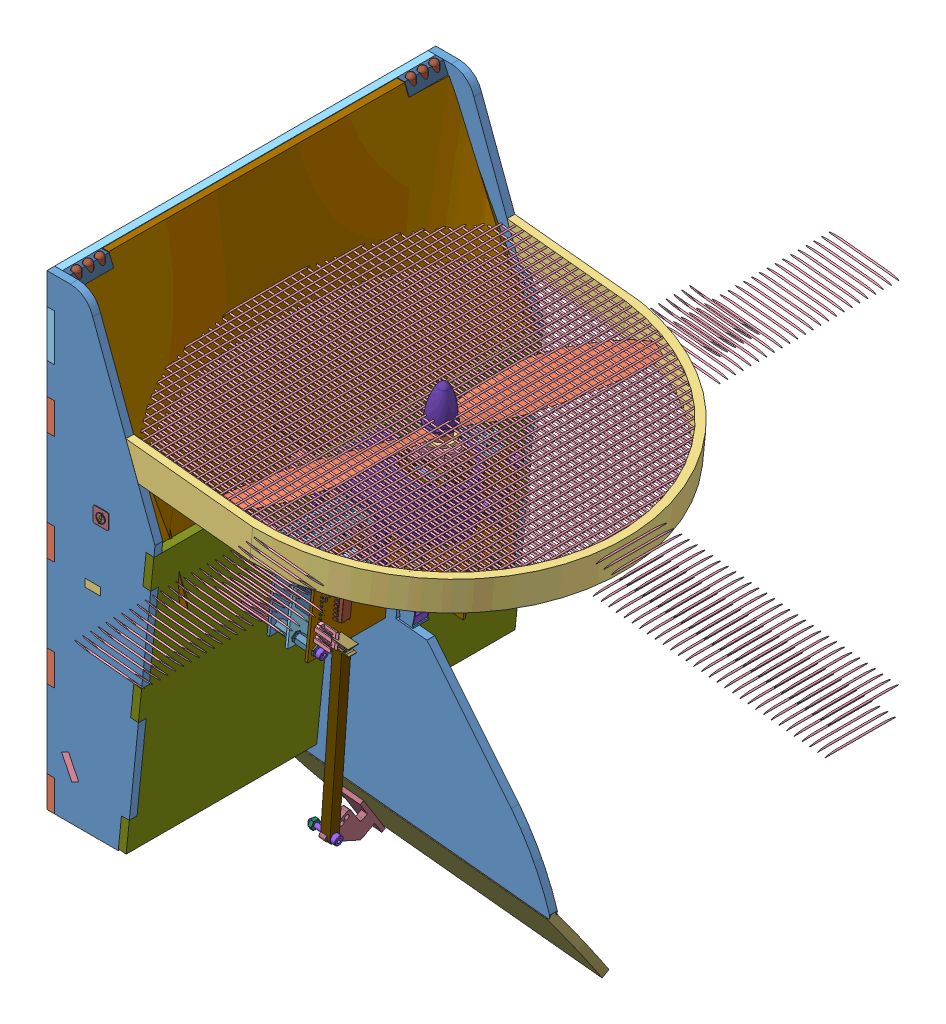
SolidWorks assembly AssTotaleSimu6, configuration Défaut. Lengths in mm. (continued)
Components (placement in the parent): (continued)
- AssStructSimu-1: AssStructSimu [Défaut] at (-125.7658 -1.8483 624.6548) x (1 0 0) z (0 0 -1) size (253.25 324.59 251.6) (continued)
  - AssProtec-1: AssProtec [Défaut] at (86.6746 190.4649 284.6351) x (0 0 -1) z (0.101852 -0.9948 0) size (250 237.46 20) (continued)
    - AssGrillage-2: AssGrillage [Défaut] at (339.6086 -132.5428 241.6839) x (0 0 1) z (-1 0 0) size (2.02 237.05 250) (continued)
      - barreau-208: barreau [Défaut] at (-0.1839 -1.5314 233.7823) x (0.998922 0 0.04641) z (0 1 0) size (1 1 400)
      - barreau-209: barreau [Défaut] at (-0.1839 -1.5314 228.7823) x (0.998922 0 0.04641) z (0 1 0) size (1 1 400)
      - barreau-210: barreau [Défaut] at (-0.1839 -1.5314 223.7823) x (0.998922 0 0.04641) z (0 1 0) size (1 1 400)
      - barreau-211: barreau [Défaut] at (-0.1839 -1.5314 218.7823) x (0.998922 0 0.04641) z (0 1 0) size (1 1 400)
      - barreau-212: barreau [Défaut] at (-0.1839 -1.5314 213.7823) x (0.998922 0 0.04641) z (0 1 0) size (1 1 400)
      - barreau-213: barreau [Défaut] at (-0.1839 -1.5314 208.7823) x (0.998922 0 0.04641) z (0 1 0) size (1 1 400)
      - barreau-214: barreau [Défaut] at (-0.1839 -1.5314 203.7823) x (0.998922 0 0.04641) z (0 1 0) size (1 1 400)
  - AssCarte-1: AssCarte [Défaut] at (38.0121 147.1029 290.772) x (-0.101852 0.9948 0) z (0.9948 0.101852 0) size (66.52 130.57 98.72)
    - carte_onduleur_v3-1: carte_onduleur_v3 [Défaut] at (-131.8199 12.0892 20.7912) size (66.52 130.57 82.34)
      - Layer_1-1: Layer_1 [Défaut] at origin size (60 130 1.61)
      - BTN-1: BTN [Défaut] at (-25.5 7.4 0.803) x (0 -1 0) z (0 0 1) size (6.76 3.64 4.37)
        - Open CASCADE STEP translator 6.8 1.2.1-1: Open CASCADE STEP translator 6.8 1.2.1 [Défaut] at origin size (6.76 3.64 4.37)
          - Body_1-1: Body_1 [Défaut] at (-0.5 -2 0) size (6.76 3.64 4.37)
            - =_[0_1_1_3]-1: =_[0_1_1_3] [Défaut] at origin size (6 3.64 4.37)
            - =_[0_1_1_4]-1: =_[0_1_1_4] [Défaut] at origin size (0.38 1 0.67)
            - =_[0_1_1_5]-1: =_[0_1_1_5] [Défaut] at origin size (0.38 1 0.67)
      - CON_IO1-1: CON_IO1 [Défaut] at (-11.3 12.1 0.803) x (0 -1 0) z (0 0 1) size (13 30 57.5)
        - Open CASCADE STEP translator 6.8 1.3.1-1: Open CASCADE STEP translator 6.8 1.3.1 [Défaut] at origin size (13 30 57.5)
          - Body_1_2-1: Body_1_2 [Défaut] at (-3 -15 8) x (0 -1 0) z (-1 0 0) size (30 57.5 13)
            - 1-1: 1 [Défaut] at origin size (30 50 1.61)
            - 10-1: 10 [Défaut] at (-14.395 31.0465 0.803) x (-1 0 0) z (0 0 1) size (5.59 6.35 1.11)
              - =_[0_1_1_4]-1: =_[0_1_1_4] [Défaut] at origin size (5.59 6.35 1.11)
                - 11-1: 11 [Défaut] at (2 3.3 0) x (-1 0 0) z (0 0 1) size (5.59 6.35 1.11)
                  - =_[0_1_1_3]_2-1: =_[0_1_1_3]_2 [Défaut] at origin size (0.44 0.55 0.36)
                  - =_[0_1_1_4]_2-1: =_[0_1_1_4]_2 [Défaut] at origin size (5.59 4.15 0.36)
                  - =_[0_1_1_5]_2-1: =_[0_1_1_5]_2 [Défaut] at origin size (5.35 6.1 1.1)
                  - =_[0_1_1_6]-1: =_[0_1_1_6] [Défaut] at origin size (0.44 0.55 0.36)
                  - =_[0_1_1_7]-1: =_[0_1_1_7] [Défaut] at origin size (0.44 0.55 0.36)
                  - =_[0_1_1_8]-1: =_[0_1_1_8] [Défaut] at origin size (0.44 0.55 0.36)
            - 13-1: 13 [Défaut] at (-12.62 16.6 -0.803) x (-1 0 0) z (0 0 -1) size (5.59 6.35 1.11)
              - =_[0_1_1_13]-1: =_[0_1_1_13] [Défaut] at origin size (5.59 6.35 1.11)
                - 11-1: 11 [Défaut] at (2 3.3 0) x (-1 0 0) z (0 0 1) size (5.59 6.35 1.11)
                  - =_[0_1_1_3]_2-1: =_[0_1_1_3]_2 [Défaut] at origin size (0.44 0.55 0.36)
                  - =_[0_1_1_4]_2-1: =_[0_1_1_4]_2 [Défaut] at origin size (5.59 4.15 0.36)
                  - =_[0_1_1_5]_2-1: =_[0_1_1_5]_2 [Défaut] at origin size (5.35 6.1 1.1)
                  - =_[0_1_1_6]-1: =_[0_1_1_6] [Défaut] at origin size (0.44 0.55 0.36)
                  - =_[0_1_1_7]-1: =_[0_1_1_7] [Défaut] at origin size (0.44 0.55 0.36)
                  - =_[0_1_1_8]-1: =_[0_1_1_8] [Défaut] at origin size (0.44 0.55 0.36)
            - 16-1: 16 [Défaut] at (-4.2 24.2 0.803) x (-1 0 0) z (0 0 1) size (12.8 0.5 13)
              - =_[0_1_1_15]-1: =_[0_1_1_15] [Défaut] at origin size (12.8 0.5 13)
                - 17-1: 17 [Défaut] at (2.7 0 0) x (1 0 0) z (0 -1 0) size (12.8 13 0.5)
            - 19-1: 19 [Défaut] at (-4.1 6.8 0.803) x (-1 0 0) z (0 0 1) size (12.8 0.5 13)
              - =_[0_1_1_18]-1: =_[0_1_1_18] [Défaut] at origin size (12.8 0.5 13)
                - 17-1: 17 [Défaut] at (2.7 0 0) x (1 0 0) z (0 -1 0) size (12.8 13 0.5)
            - 24-1: 24 [Défaut] at (-8.1 16.5 -0.803) x (0 1 0) z (0 0 -1) size (7.75 5.13 1.17)
              - =_[0_1_1_20]-1: =_[0_1_1_20] [Défaut] at origin size (7.75 5.13 1.17)
                - 20-1: 20 [Défaut] at origin size (7.59 5.13 1.07)
                - 21-1: 21 [Défaut] at (-14.478 0 0) x (-1 0 0) z (0 0 1) size (0.76 5.08 1.17)
                - 22-1: 22 [Défaut] at origin size (0.76 5.08 1.17)
            - 35-1: 35 [Défaut] at (-25.3 25.5 0.803) x (0 -1 0) z (0 0 1) size (6.05 5.2 1.7)
              - =_[0_1_1_25]-1: =_[0_1_1_25] [Défaut] at origin size (6.05 5.2 1.7)
                - 25-1: 25 [Défaut] at origin size (4.3 5.2 1.53)
                - 26-1: 26 [Défaut] at origin size (0.88 0.51 1.06)
                - 27-1: 27 [Défaut] at origin size (0.88 0.51 1.06)
                - 28-1: 28 [Défaut] at origin size (0.88 0.51 1.06)
                - 29-1: 29 [Défaut] at origin size (0.88 0.51 1.06)
                - 30-1: 30 [Défaut] at (11.6 -5.08 0) x (-1 0 0) z (0 0 1) size (0.87 0.51 1.06)
                - 31-1: 31 [Défaut] at (11.6 -2.54 0) x (-1 0 0) z (0 0 1) size (0.87 0.51 1.06)
                - 32-1: 32 [Défaut] at (11.6 0 0) x (-1 0 0) z (0 0 1) size (0.87 0.51 1.06)
                - 33-1: 33 [Défaut] at (11.6 2.54 0) x (-1 0 0) z (0 0 1) size (0.87 0.51 1.06)
            - 40-1: 40 [Défaut] at (-27.6 27.2 0.803) size (2.34 1.04 0.5)
              - =_[0_1_1_36]-1: =_[0_1_1_36] [Défaut] at origin size (2.34 1.04 0.5)
                - 36-1: 36 [Défaut] at origin size (2.29 1.04 0.43)
                - 37-1: 37 [Défaut] at (0.3048 0 0) x (-1 0 0) z (0 0 1) size (0.51 1.02 0.5)
                - 38-1: 38 [Défaut] at origin size (0.51 1.02 0.5)
            - 42-1: 42 [Défaut] at (-22.1 21.6 0.803) x (0 1 0) z (0 0 1) size (2.34 1.04 0.5)
              - =_[0_1_1_36]-1: =_[0_1_1_36] [Défaut] at origin size (2.34 1.04 0.5)
                - 36-1: 36 [Défaut] at origin size (2.29 1.04 0.43)
                - 37-1: 37 [Défaut] at (0.3048 0 0) x (-1 0 0) z (0 0 1) size (0.51 1.02 0.5)
                - 38-1: 38 [Défaut] at origin size (0.51 1.02 0.5)
            - 47-1: 47 [Défaut] at (-14.7664 14.5 -0.803) x (-1 0 0) z (0 0 -1) size (2.34 1.04 0.5)
              - =_[0_1_1_42]-1: =_[0_1_1_42] [Défaut] at origin size (2.34 1.04 0.5)
                - 43-1: 43 [Défaut] at origin size (2.29 1.04 0.43)
                - 44-1: 44 [Défaut] at (0.3048 0 0) x (-1 0 0) z (0 0 1) size (0.51 1.02 0.5)
                - 45-1: 45 [Défaut] at origin size (0.51 1.02 0.5)
            - 57-1: 57 [Défaut] at (-15.3 2.7 -0.803) x (0 -1 0) z (0 0 -1) size (10.36 15.24 6.14)
              - =_[0_1_1_47]-1: =_[0_1_1_47] [Défaut] at origin size (10.36 15.24 6.14)
                - 55-1: 55 [Défaut] at (1.8 -1.2 3) x (1 0 0) z (0 1 0) size (10.36 6.14 15.24)
                  - 54-1: 54 [Défaut] at origin size (10.36 6.14 7.62)
                    - 52-1: 52 [Défaut] at origin size (10.36 6.14 2.54)
                      - 48-1: 48 [Défaut] at origin size (8.4 2.54 2.54)
                      - 49-1: 49 [Défaut] at (-0.0461 1.2682 1.27) x (0 0 -1) z (0.999998 -0.002105 0) size (1.95 5.07 7.58)
                    - 52-2: 52 [Défaut] at (0 0 -2.54) size (10.36 6.14 2.54)
                      - 48-1: 48 [Défaut] at origin size (8.4 2.54 2.54)
                      - 49-1: 49 [Défaut] at (-0.0461 1.2682 1.27) x (0 0 -1) z (0.999998 -0.002105 0) size (1.95 5.07 7.58)
                    - 52-3: 52 [Défaut] at (0 0 -5.08) size (10.36 6.14 2.54)
                      - 48-1: 48 [Défaut] at origin size (8.4 2.54 2.54)
                      - 49-1: 49 [Défaut] at (-0.0461 1.2682 1.27) x (0 0 -1) z (0.999998 -0.002105 0) size (1.95 5.07 7.58)
                  - 54-2: 54 [Défaut] at (0 0 -7.62) size (10.36 6.14 7.62)
                    - 52-1: 52 [Défaut] at origin size (10.36 6.14 2.54)
                      - 48-1: 48 [Défaut] at origin size (8.4 2.54 2.54)
                      - 49-1: 49 [Défaut] at (-0.0461 1.2682 1.27) x (0 0 -1) z (0.999998 -0.002105 0) size (1.95 5.07 7.58)
                    - 52-2: 52 [Défaut] at (0 0 -2.54) size (10.36 6.14 2.54)
                      - 48-1: 48 [Défaut] at origin size (8.4 2.54 2.54)
                      - 49-1: 49 [Défaut] at (-0.0461 1.2682 1.27) x (0 0 -1) z (0.999998 -0.002105 0) size (1.95 5.07 7.58)
                    - 52-3: 52 [Défaut] at (0 0 -5.08) size (10.36 6.14 2.54)
                      - 48-1: 48 [Défaut] at origin size (8.4 2.54 2.54)
                      - 49-1: 49 [Défaut] at (-0.0461 1.2682 1.27) x (0 0 -1) z (0.999998 -0.002105 0) size (1.95 5.07 7.58)
            - 59-1: 59 [Défaut] at (-26.5 31 0.803) x (0 -1 0) z (0 0 1) size (2.34 1.04 0.5)
              - =_[0_1_1_42]-1: =_[0_1_1_42] [Défaut] at origin size (2.34 1.04 0.5)
                - 43-1: 43 [Défaut] at origin size (2.29 1.04 0.43)
                - 44-1: 44 [Défaut] at (0.3048 0 0) x (-1 0 0) z (0 0 1) size (0.51 1.02 0.5)
                - 45-1: 45 [Défaut] at origin size (0.51 1.02 0.5)
            - 61-1: 61 [Défaut] at (-21.6 17.8 0.803) x (-1 0 0) z (0 0 1) size (2.34 1.04 0.5)
              - =_[0_1_1_42]-1: =_[0_1_1_42] [Défaut] at origin size (2.34 1.04 0.5)
                - 43-1: 43 [Défaut] at origin size (2.29 1.04 0.43)
                - 44-1: 44 [Défaut] at (0.3048 0 0) x (-1 0 0) z (0 0 1) size (0.51 1.02 0.5)
                - 45-1: 45 [Défaut] at origin size (0.51 1.02 0.5)
            - 74-1: 74 [Défaut] at (-4.9 41.8 0.803) x (0 -1 0) z (0 0 1) size (6 4.9 1.75)
              - =_[0_1_1_56]-1: =_[0_1_1_56] [Défaut] at origin size (6 4.9 1.75)
                - 72-1: 72 [Défaut] at origin size (6 4.9 1.75)
                  - =_[0_1_1_2]-1: =_[0_1_1_2] [Défaut] at origin size (3.9 4.9 1.57)
                  - =_[0_1_1_3]-1: =_[0_1_1_3] [Défaut] at origin size (6 4.22 1)
                    - =_[0_1_1_60]-1: =_[0_1_1_60] [Défaut] at origin size (1.05 0.41 1)
                    - =_[0_1_1_61]-1: =_[0_1_1_61] [Défaut] at origin size (1.05 0.41 1)
                    - =_[0_1_1_62]-1: =_[0_1_1_62] [Défaut] at origin size (1.05 0.41 1)
                    - =_[0_1_1_63]-1: =_[0_1_1_63] [Défaut] at origin size (1.05 0.41 1)
                    - =_[0_1_1_64]-1: =_[0_1_1_64] [Défaut] at origin size (1.05 0.41 1)
                    - =_[0_1_1_65]-1: =_[0_1_1_65] [Défaut] at origin size (1.05 0.41 1)
                    - =_[0_1_1_66]-1: =_[0_1_1_66] [Défaut] at origin size (1.05 0.41 1)
                    - =_[0_1_1_67]-1: =_[0_1_1_67] [Défaut] at origin size (1.05 0.41 1)
            - 76-1: 76 [Défaut] at (-8.5 40.5664 0.803) x (0 1 0) z (0 0 1) size (2.34 1.04 0.5)
              - =_[0_1_1_42]-1: =_[0_1_1_42] [Défaut] at origin size (2.34 1.04 0.5)
                - 43-1: 43 [Défaut] at origin size (2.29 1.04 0.43)
                - 44-1: 44 [Défaut] at (0.3048 0 0) x (-1 0 0) z (0 0 1) size (0.51 1.02 0.5)
                - 45-1: 45 [Défaut] at origin size (0.51 1.02 0.5)
            - 78-1: 78 [Défaut] at (-5.9 46.4 0.803) x (-1 0 0) z (0 0 1) size (2.34 1.04 0.5)
              - =_[0_1_1_42]-1: =_[0_1_1_42] [Défaut] at origin size (2.34 1.04 0.5)
                - 43-1: 43 [Défaut] at origin size (2.29 1.04 0.43)
                - 44-1: 44 [Défaut] at (0.3048 0 0) x (-1 0 0) z (0 0 1) size (0.51 1.02 0.5)
                - 45-1: 45 [Défaut] at origin size (0.51 1.02 0.5)
            - 80-1: 80 [Défaut] at (-7 48.1 0.803) size (2.34 1.04 0.5)
              - =_[0_1_1_42]-1: =_[0_1_1_42] [Défaut] at origin size (2.34 1.04 0.5)
                - 43-1: 43 [Défaut] at origin size (2.29 1.04 0.43)
                - 44-1: 44 [Défaut] at (0.3048 0 0) x (-1 0 0) z (0 0 1) size (0.51 1.02 0.5)
                - 45-1: 45 [Défaut] at origin size (0.51 1.02 0.5)
            - 82-1: 82 [Défaut] at (-6 37.1 0.803) size (2.34 1.04 0.5)
              - =_[0_1_1_42]-1: =_[0_1_1_42] [Défaut] at origin size (2.34 1.04 0.5)
                - 43-1: 43 [Défaut] at origin size (2.29 1.04 0.43)
                - 44-1: 44 [Défaut] at (0.3048 0 0) x (-1 0 0) z (0 0 1) size (0.51 1.02 0.5)
                - 45-1: 45 [Défaut] at origin size (0.51 1.02 0.5)
      - CON_IO2-1: CON_IO2 [Défaut] at (-11.3 -2.7 0.803) x (0 -1 0) z (0 0 1) size (13 30 57.5)
        - Open CASCADE STEP translator 6.8 1.4.1-1: Open CASCADE STEP translator 6.8 1.4.1 [Défaut] at origin size (13 30 57.5)
          - Body_1_2-1: Body_1_2 [Défaut] at (-3 -15 8) x (0 -1 0) z (-1 0 0) size (30 57.5 13)
            - 1-1: 1 [Défaut] at origin size (30 50 1.61)
            - 10-1: 10 [Défaut] at (-14.395 31.0465 0.803) x (-1 0 0) z (0 0 1) size (5.59 6.35 1.11)
              - =_[0_1_1_4]-1: =_[0_1_1_4] [Défaut] at origin size (5.59 6.35 1.11)
                - 11-1: 11 [Défaut] at (2 3.3 0) x (-1 0 0) z (0 0 1) size (5.59 6.35 1.11)
                  - =_[0_1_1_3]_2-1: =_[0_1_1_3]_2 [Défaut] at origin size (0.44 0.55 0.36)
                  - =_[0_1_1_4]_2-1: =_[0_1_1_4]_2 [Défaut] at origin size (5.59 4.15 0.36)
                  - =_[0_1_1_5]_2-1: =_[0_1_1_5]_2 [Défaut] at origin size (5.35 6.1 1.1)
                  - =_[0_1_1_6]-1: =_[0_1_1_6] [Défaut] at origin size (0.44 0.55 0.36)
                  - =_[0_1_1_7]-1: =_[0_1_1_7] [Défaut] at origin size (0.44 0.55 0.36)
                  - =_[0_1_1_8]-1: =_[0_1_1_8] [Défaut] at origin size (0.44 0.55 0.36)
            - 13-1: 13 [Défaut] at (-12.62 16.6 -0.803) x (-1 0 0) z (0 0 -1) size (5.59 6.35 1.11)
              - =_[0_1_1_13]-1: =_[0_1_1_13] [Défaut] at origin size (5.59 6.35 1.11)
                - 11-1: 11 [Défaut] at (2 3.3 0) x (-1 0 0) z (0 0 1) size (5.59 6.35 1.11)
                  - =_[0_1_1_3]_2-1: =_[0_1_1_3]_2 [Défaut] at origin size (0.44 0.55 0.36)
                  - =_[0_1_1_4]_2-1: =_[0_1_1_4]_2 [Défaut] at origin size (5.59 4.15 0.36)
                  - =_[0_1_1_5]_2-1: =_[0_1_1_5]_2 [Défaut] at origin size (5.35 6.1 1.1)
                  - =_[0_1_1_6]-1: =_[0_1_1_6] [Défaut] at origin size (0.44 0.55 0.36)
                  - =_[0_1_1_7]-1: =_[0_1_1_7] [Défaut] at origin size (0.44 0.55 0.36)
                  - =_[0_1_1_8]-1: =_[0_1_1_8] [Défaut] at origin size (0.44 0.55 0.36)
            - 16-1: 16 [Défaut] at (-4.2 24.2 0.803) x (-1 0 0) z (0 0 1) size (12.8 0.5 13)
              - =_[0_1_1_15]-1: =_[0_1_1_15] [Défaut] at origin size (12.8 0.5 13)
                - 17-1: 17 [Défaut] at (2.7 0 0) x (1 0 0) z (0 -1 0) size (12.8 13 0.5)
            - 19-1: 19 [Défaut] at (-4.1 6.8 0.803) x (-1 0 0) z (0 0 1) size (12.8 0.5 13)
              - =_[0_1_1_18]-1: =_[0_1_1_18] [Défaut] at origin size (12.8 0.5 13)
                - 17-1: 17 [Défaut] at (2.7 0 0) x (1 0 0) z (0 -1 0) size (12.8 13 0.5)
            - 24-1: 24 [Défaut] at (-8.1 16.5 -0.803) x (0 1 0) z (0 0 -1) size (7.75 5.13 1.17)
              - =_[0_1_1_20]-1: =_[0_1_1_20] [Défaut] at origin size (7.75 5.13 1.17)
                - 20-1: 20 [Défaut] at origin size (7.59 5.13 1.07)
                - 21-1: 21 [Défaut] at (-14.478 0 0) x (-1 0 0) z (0 0 1) size (0.76 5.08 1.17)
                - 22-1: 22 [Défaut] at origin size (0.76 5.08 1.17)
            - 35-1: 35 [Défaut] at (-25.3 25.5 0.803) x (0 -1 0) z (0 0 1) size (6.05 5.2 1.7)
              - =_[0_1_1_25]-1: =_[0_1_1_25] [Défaut] at origin size (6.05 5.2 1.7)
                - 25-1: 25 [Défaut] at origin size (4.3 5.2 1.53)
                - 26-1: 26 [Défaut] at origin size (0.88 0.51 1.06)
                - 27-1: 27 [Défaut] at origin size (0.88 0.51 1.06)
                - 28-1: 28 [Défaut] at origin size (0.88 0.51 1.06)
                - 29-1: 29 [Défaut] at origin size (0.88 0.51 1.06)
                - 30-1: 30 [Défaut] at (11.6 -5.08 0) x (-1 0 0) z (0 0 1) size (0.87 0.51 1.06)
                - 31-1: 31 [Défaut] at (11.6 -2.54 0) x (-1 0 0) z (0 0 1) size (0.87 0.51 1.06)
                - 32-1: 32 [Défaut] at (11.6 0 0) x (-1 0 0) z (0 0 1) size (0.87 0.51 1.06)
                - 33-1: 33 [Défaut] at (11.6 2.54 0) x (-1 0 0) z (0 0 1) size (0.87 0.51 1.06)
            - 40-1: 40 [Défaut] at (-27.6 27.2 0.803) size (2.34 1.04 0.5)
              - =_[0_1_1_36]-1: =_[0_1_1_36] [Défaut] at origin size (2.34 1.04 0.5)
                - 36-1: 36 [Défaut] at origin size (2.29 1.04 0.43)
                - 37-1: 37 [Défaut] at (0.3048 0 0) x (-1 0 0) z (0 0 1) size (0.51 1.02 0.5)
                - 38-1: 38 [Défaut] at origin size (0.51 1.02 0.5)
            - 42-1: 42 [Défaut] at (-22.1 21.6 0.803) x (0 1 0) z (0 0 1) size (2.34 1.04 0.5)
              - =_[0_1_1_36]-1: =_[0_1_1_36] [Défaut] at origin size (2.34 1.04 0.5)
                - 36-1: 36 [Défaut] at origin size (2.29 1.04 0.43)
                - 37-1: 37 [Défaut] at (0.3048 0 0) x (-1 0 0) z (0 0 1) size (0.51 1.02 0.5)
                - 38-1: 38 [Défaut] at origin size (0.51 1.02 0.5)
            - 47-1: 47 [Défaut] at (-14.7664 14.5 -0.803) x (-1 0 0) z (0 0 -1) size (2.34 1.04 0.5)
              - =_[0_1_1_42]-1: =_[0_1_1_42] [Défaut] at origin size (2.34 1.04 0.5)
                - 43-1: 43 [Défaut] at origin size (2.29 1.04 0.43)
                - 44-1: 44 [Défaut] at (0.3048 0 0) x (-1 0 0) z (0 0 1) size (0.51 1.02 0.5)
                - 45-1: 45 [Défaut] at origin size (0.51 1.02 0.5)
            - 57-1: 57 [Défaut] at (-15.3 2.7 -0.803) x (0 -1 0) z (0 0 -1) size (10.36 15.24 6.14)
              - =_[0_1_1_47]-1: =_[0_1_1_47] [Défaut] at origin size (10.36 15.24 6.14)
                - 55-1: 55 [Défaut] at (1.8 -1.2 3) x (1 0 0) z (0 1 0) size (10.36 6.14 15.24)
                  - 54-1: 54 [Défaut] at origin size (10.36 6.14 7.62)
                    - 52-1: 52 [Défaut] at origin size (10.36 6.14 2.54)
                      - 48-1: 48 [Défaut] at origin size (8.4 2.54 2.54)
                      - 49-1: 49 [Défaut] at (-0.0461 1.2682 1.27) x (0 0 -1) z (0.999998 -0.002105 0) size (1.95 5.07 7.58)
                    - 52-2: 52 [Défaut] at (0 0 -2.54) size (10.36 6.14 2.54)
                      - 48-1: 48 [Défaut] at origin size (8.4 2.54 2.54)
                      - 49-1: 49 [Défaut] at (-0.0461 1.2682 1.27) x (0 0 -1) z (0.999998 -0.002105 0) size (1.95 5.07 7.58)
                    - 52-3: 52 [Défaut] at (0 0 -5.08) size (10.36 6.14 2.54)
                      - 48-1: 48 [Défaut] at origin size (8.4 2.54 2.54)
                      - 49-1: 49 [Défaut] at (-0.0461 1.2682 1.27) x (0 0 -1) z (0.999998 -0.002105 0) size (1.95 5.07 7.58)
                  - 54-2: 54 [Défaut] at (0 0 -7.62) size (10.36 6.14 7.62)
                    - 52-1: 52 [Défaut] at origin size (10.36 6.14 2.54)
                      - 48-1: 48 [Défaut] at origin size (8.4 2.54 2.54)
                      - 49-1: 49 [Défaut] at (-0.0461 1.2682 1.27) x (0 0 -1) z (0.999998 -0.002105 0) size (1.95 5.07 7.58)
                    - 52-2: 52 [Défaut] at (0 0 -2.54) size (10.36 6.14 2.54)
                      - 48-1: 48 [Défaut] at origin size (8.4 2.54 2.54)
                      - 49-1: 49 [Défaut] at (-0.0461 1.2682 1.27) x (0 0 -1) z (0.999998 -0.002105 0) size (1.95 5.07 7.58)
                    - 52-3: 52 [Défaut] at (0 0 -5.08) size (10.36 6.14 2.54)
                      - 48-1: 48 [Défaut] at origin size (8.4 2.54 2.54)
                      - 49-1: 49 [Défaut] at (-0.0461 1.2682 1.27) x (0 0 -1) z (0.999998 -0.002105 0) size (1.95 5.07 7.58)
            - 59-1: 59 [Défaut] at (-26.5 31 0.803) x (0 -1 0) z (0 0 1) size (2.34 1.04 0.5)
              - =_[0_1_1_42]-1: =_[0_1_1_42] [Défaut] at origin size (2.34 1.04 0.5)
                - 43-1: 43 [Défaut] at origin size (2.29 1.04 0.43)
                - 44-1: 44 [Défaut] at (0.3048 0 0) x (-1 0 0) z (0 0 1) size (0.51 1.02 0.5)
                - 45-1: 45 [Défaut] at origin size (0.51 1.02 0.5)
            - 61-1: 61 [Défaut] at (-21.6 17.8 0.803) x (-1 0 0) z (0 0 1) size (2.34 1.04 0.5)
              - =_[0_1_1_42]-1: =_[0_1_1_42] [Défaut] at origin size (2.34 1.04 0.5)
                - 43-1: 43 [Défaut] at origin size (2.29 1.04 0.43)
                - 44-1: 44 [Défaut] at (0.3048 0 0) x (-1 0 0) z (0 0 1) size (0.51 1.02 0.5)
                - 45-1: 45 [Défaut] at origin size (0.51 1.02 0.5)
            - 74-1: 74 [Défaut] at (-4.9 41.8 0.803) x (0 -1 0) z (0 0 1) size (6 4.9 1.75)
              - =_[0_1_1_56]-1: =_[0_1_1_56] [Défaut] at origin size (6 4.9 1.75)
                - 72-1: 72 [Défaut] at origin size (6 4.9 1.75)
                  - =_[0_1_1_2]-1: =_[0_1_1_2] [Défaut] at origin size (3.9 4.9 1.57)
                  - =_[0_1_1_3]-1: =_[0_1_1_3] [Défaut] at origin size (6 4.22 1)
                    - =_[0_1_1_60]-1: =_[0_1_1_60] [Défaut] at origin size (1.05 0.41 1)
                    - =_[0_1_1_61]-1: =_[0_1_1_61] [Défaut] at origin size (1.05 0.41 1)
                    - =_[0_1_1_62]-1: =_[0_1_1_62] [Défaut] at origin size (1.05 0.41 1)
                    - =_[0_1_1_63]-1: =_[0_1_1_63] [Défaut] at origin size (1.05 0.41 1)
                    - =_[0_1_1_64]-1: =_[0_1_1_64] [Défaut] at origin size (1.05 0.41 1)
                    - =_[0_1_1_65]-1: =_[0_1_1_65] [Défaut] at origin size (1.05 0.41 1)
                    - =_[0_1_1_66]-1: =_[0_1_1_66] [Défaut] at origin size (1.05 0.41 1)
                    - =_[0_1_1_67]-1: =_[0_1_1_67] [Défaut] at origin size (1.05 0.41 1)
            - 76-1: 76 [Défaut] at (-8.5 40.5664 0.803) x (0 1 0) z (0 0 1) size (2.34 1.04 0.5)
              - =_[0_1_1_42]-1: =_[0_1_1_42] [Défaut] at origin size (2.34 1.04 0.5)
                - 43-1: 43 [Défaut] at origin size (2.29 1.04 0.43)
                - 44-1: 44 [Défaut] at (0.3048 0 0) x (-1 0 0) z (0 0 1) size (0.51 1.02 0.5)
                - 45-1: 45 [Défaut] at origin size (0.51 1.02 0.5)
            - 78-1: 78 [Défaut] at (-5.9 46.4 0.803) x (-1 0 0) z (0 0 1) size (2.34 1.04 0.5)
              - =_[0_1_1_42]-1: =_[0_1_1_42] [Défaut] at origin size (2.34 1.04 0.5)
                - 43-1: 43 [Défaut] at origin size (2.29 1.04 0.43)
                - 44-1: 44 [Défaut] at (0.3048 0 0) x (-1 0 0) z (0 0 1) size (0.51 1.02 0.5)
                - 45-1: 45 [Défaut] at origin size (0.51 1.02 0.5)
            - 80-1: 80 [Défaut] at (-7 48.1 0.803) size (2.34 1.04 0.5)
              - =_[0_1_1_42]-1: =_[0_1_1_42] [Défaut] at origin size (2.34 1.04 0.5)
                - 43-1: 43 [Défaut] at origin size (2.29 1.04 0.43)
                - 44-1: 44 [Défaut] at (0.3048 0 0) x (-1 0 0) z (0 0 1) size (0.51 1.02 0.5)
                - 45-1: 45 [Défaut] at origin size (0.51 1.02 0.5)
            - 82-1: 82 [Défaut] at (-6 37.1 0.803) size (2.34 1.04 0.5)
              - =_[0_1_1_42]-1: =_[0_1_1_42] [Défaut] at origin size (2.34 1.04 0.5)
                - 43-1: 43 [Défaut] at origin size (2.29 1.04 0.43)
                - 44-1: 44 [Défaut] at (0.3048 0 0) x (-1 0 0) z (0 0 1) size (0.51 1.02 0.5)
                - 45-1: 45 [Défaut] at origin size (0.51 1.02 0.5)
      - CON_IO3-1: CON_IO3 [Défaut] at (-11.3 -17.7 0.803) x (0 -1 0) z (0 0 1) size (13 30 57.5)
        - Open CASCADE STEP translator 6.8 1.5.1-1: Open CASCADE STEP translator 6.8 1.5.1 [Défaut] at origin size (13 30 57.5)
          - Body_1_2-1: Body_1_2 [Défaut] at (-3 -15 8) x (0 -1 0) z (-1 0 0) size (30 57.5 13)
            - 1-1: 1 [Défaut] at origin size (30 50 1.61)
            - 10-1: 10 [Défaut] at (-14.395 31.0465 0.803) x (-1 0 0) z (0 0 1) size (5.59 6.35 1.11)
              - =_[0_1_1_4]-1: =_[0_1_1_4] [Défaut] at origin size (5.59 6.35 1.11)
                - 11-1: 11 [Défaut] at (2 3.3 0) x (-1 0 0) z (0 0 1) size (5.59 6.35 1.11)
                  - =_[0_1_1_3]_2-1: =_[0_1_1_3]_2 [Défaut] at origin size (0.44 0.55 0.36)
                  - =_[0_1_1_4]_2-1: =_[0_1_1_4]_2 [Défaut] at origin size (5.59 4.15 0.36)
                  - =_[0_1_1_5]_2-1: =_[0_1_1_5]_2 [Défaut] at origin size (5.35 6.1 1.1)
                  - =_[0_1_1_6]-1: =_[0_1_1_6] [Défaut] at origin size (0.44 0.55 0.36)
                  - =_[0_1_1_7]-1: =_[0_1_1_7] [Défaut] at origin size (0.44 0.55 0.36)
                  - =_[0_1_1_8]-1: =_[0_1_1_8] [Défaut] at origin size (0.44 0.55 0.36)
            - 13-1: 13 [Défaut] at (-12.62 16.6 -0.803) x (-1 0 0) z (0 0 -1) size (5.59 6.35 1.11)
              - =_[0_1_1_13]-1: =_[0_1_1_13] [Défaut] at origin size (5.59 6.35 1.11)
                - 11-1: 11 [Défaut] at (2 3.3 0) x (-1 0 0) z (0 0 1) size (5.59 6.35 1.11)
                  - =_[0_1_1_3]_2-1: =_[0_1_1_3]_2 [Défaut] at origin size (0.44 0.55 0.36)
                  - =_[0_1_1_4]_2-1: =_[0_1_1_4]_2 [Défaut] at origin size (5.59 4.15 0.36)
                  - =_[0_1_1_5]_2-1: =_[0_1_1_5]_2 [Défaut] at origin size (5.35 6.1 1.1)
                  - =_[0_1_1_6]-1: =_[0_1_1_6] [Défaut] at origin size (0.44 0.55 0.36)
                  - =_[0_1_1_7]-1: =_[0_1_1_7] [Défaut] at origin size (0.44 0.55 0.36)
                  - =_[0_1_1_8]-1: =_[0_1_1_8] [Défaut] at origin size (0.44 0.55 0.36)
            - 16-1: 16 [Défaut] at (-4.2 24.2 0.803) x (-1 0 0) z (0 0 1) size (12.8 0.5 13)
              - =_[0_1_1_15]-1: =_[0_1_1_15] [Défaut] at origin size (12.8 0.5 13)
                - 17-1: 17 [Défaut] at (2.7 0 0) x (1 0 0) z (0 -1 0) size (12.8 13 0.5)
            - 19-1: 19 [Défaut] at (-4.1 6.8 0.803) x (-1 0 0) z (0 0 1) size (12.8 0.5 13)
              - =_[0_1_1_18]-1: =_[0_1_1_18] [Défaut] at origin size (12.8 0.5 13)
                - 17-1: 17 [Défaut] at (2.7 0 0) x (1 0 0) z (0 -1 0) size (12.8 13 0.5)
            - 24-1: 24 [Défaut] at (-8.1 16.5 -0.803) x (0 1 0) z (0 0 -1) size (7.75 5.13 1.17)
              - =_[0_1_1_20]-1: =_[0_1_1_20] [Défaut] at origin size (7.75 5.13 1.17)
                - 20-1: 20 [Défaut] at origin size (7.59 5.13 1.07)
                - 21-1: 21 [Défaut] at (-14.478 0 0) x (-1 0 0) z (0 0 1) size (0.76 5.08 1.17)
                - 22-1: 22 [Défaut] at origin size (0.76 5.08 1.17)
            - 35-1: 35 [Défaut] at (-25.3 25.5 0.803) x (0 -1 0) z (0 0 1) size (6.05 5.2 1.7)
              - =_[0_1_1_25]-1: =_[0_1_1_25] [Défaut] at origin size (6.05 5.2 1.7)
                - 25-1: 25 [Défaut] at origin size (4.3 5.2 1.53)
                - 26-1: 26 [Défaut] at origin size (0.88 0.51 1.06)
                - 27-1: 27 [Défaut] at origin size (0.88 0.51 1.06)
                - 28-1: 28 [Défaut] at origin size (0.88 0.51 1.06)
                - 29-1: 29 [Défaut] at origin size (0.88 0.51 1.06)
                - 30-1: 30 [Défaut] at (11.6 -5.08 0) x (-1 0 0) z (0 0 1) size (0.87 0.51 1.06)
                - 31-1: 31 [Défaut] at (11.6 -2.54 0) x (-1 0 0) z (0 0 1) size (0.87 0.51 1.06)
                - 32-1: 32 [Défaut] at (11.6 0 0) x (-1 0 0) z (0 0 1) size (0.87 0.51 1.06)
                - 33-1: 33 [Défaut] at (11.6 2.54 0) x (-1 0 0) z (0 0 1) size (0.87 0.51 1.06)
            - 40-1: 40 [Défaut] at (-27.6 27.2 0.803) size (2.34 1.04 0.5)
              - =_[0_1_1_36]-1: =_[0_1_1_36] [Défaut] at origin size (2.34 1.04 0.5)
                - 36-1: 36 [Défaut] at origin size (2.29 1.04 0.43)
                - 37-1: 37 [Défaut] at (0.3048 0 0) x (-1 0 0) z (0 0 1) size (0.51 1.02 0.5)
                - 38-1: 38 [Défaut] at origin size (0.51 1.02 0.5)
            - 42-1: 42 [Défaut] at (-22.1 21.6 0.803) x (0 1 0) z (0 0 1) size (2.34 1.04 0.5)
              - =_[0_1_1_36]-1: =_[0_1_1_36] [Défaut] at origin size (2.34 1.04 0.5)
                - 36-1: 36 [Défaut] at origin size (2.29 1.04 0.43)
                - 37-1: 37 [Défaut] at (0.3048 0 0) x (-1 0 0) z (0 0 1) size (0.51 1.02 0.5)
                - 38-1: 38 [Défaut] at origin size (0.51 1.02 0.5)
            - 47-1: 47 [Défaut] at (-14.7664 14.5 -0.803) x (-1 0 0) z (0 0 -1) size (2.34 1.04 0.5)
              - =_[0_1_1_42]-1: =_[0_1_1_42] [Défaut] at origin size (2.34 1.04 0.5)
                - 43-1: 43 [Défaut] at origin size (2.29 1.04 0.43)
                - 44-1: 44 [Défaut] at (0.3048 0 0) x (-1 0 0) z (0 0 1) size (0.51 1.02 0.5)
                - 45-1: 45 [Défaut] at origin size (0.51 1.02 0.5)
            - 57-1: 57 [Défaut] at (-15.3 2.7 -0.803) x (0 -1 0) z (0 0 -1) size (10.36 15.24 6.14)
              - =_[0_1_1_47]-1: =_[0_1_1_47] [Défaut] at origin size (10.36 15.24 6.14)
                - 55-1: 55 [Défaut] at (1.8 -1.2 3) x (1 0 0) z (0 1 0) size (10.36 6.14 15.24)
                  - 54-1: 54 [Défaut] at origin size (10.36 6.14 7.62)
                    - 52-1: 52 [Défaut] at origin size (10.36 6.14 2.54)
                      - 48-1: 48 [Défaut] at origin size (8.4 2.54 2.54)
                      - 49-1: 49 [Défaut] at (-0.0461 1.2682 1.27) x (0 0 -1) z (0.999998 -0.002105 0) size (1.95 5.07 7.58)
                    - 52-2: 52 [Défaut] at (0 0 -2.54) size (10.36 6.14 2.54)
                      - 48-1: 48 [Défaut] at origin size (8.4 2.54 2.54)
                      - 49-1: 49 [Défaut] at (-0.0461 1.2682 1.27) x (0 0 -1) z (0.999998 -0.002105 0) size (1.95 5.07 7.58)
                    - 52-3: 52 [Défaut] at (0 0 -5.08) size (10.36 6.14 2.54)
                      - 48-1: 48 [Défaut] at origin size (8.4 2.54 2.54)
                      - 49-1: 49 [Défaut] at (-0.0461 1.2682 1.27) x (0 0 -1) z (0.999998 -0.002105 0) size (1.95 5.07 7.58)
                  - 54-2: 54 [Défaut] at (0 0 -7.62) size (10.36 6.14 7.62)
                    - 52-1: 52 [Défaut] at origin size (10.36 6.14 2.54)
                      - 48-1: 48 [Défaut] at origin size (8.4 2.54 2.54)
                      - 49-1: 49 [Défaut] at (-0.0461 1.2682 1.27) x (0 0 -1) z (0.999998 -0.002105 0) size (1.95 5.07 7.58)
                    - 52-2: 52 [Défaut] at (0 0 -2.54) size (10.36 6.14 2.54)
                      - 48-1: 48 [Défaut] at origin size (8.4 2.54 2.54)
                      - 49-1: 49 [Défaut] at (-0.0461 1.2682 1.27) x (0 0 -1) z (0.999998 -0.002105 0) size (1.95 5.07 7.58)
                    - 52-3: 52 [Défaut] at (0 0 -5.08) size (10.36 6.14 2.54)
                      - 48-1: 48 [Défaut] at origin size (8.4 2.54 2.54)
                      - 49-1: 49 [Défaut] at (-0.0461 1.2682 1.27) x (0 0 -1) z (0.999998 -0.002105 0) size (1.95 5.07 7.58)
            - 59-1: 59 [Défaut] at (-26.5 31 0.803) x (0 -1 0) z (0 0 1) size (2.34 1.04 0.5)
              - =_[0_1_1_42]-1: =_[0_1_1_42] [Défaut] at origin size (2.34 1.04 0.5)
                - 43-1: 43 [Défaut] at origin size (2.29 1.04 0.43)
                - 44-1: 44 [Défaut] at (0.3048 0 0) x (-1 0 0) z (0 0 1) size (0.51 1.02 0.5)
                - 45-1: 45 [Défaut] at origin size (0.51 1.02 0.5)
            - 61-1: 61 [Défaut] at (-21.6 17.8 0.803) x (-1 0 0) z (0 0 1) size (2.34 1.04 0.5)
              - =_[0_1_1_42]-1: =_[0_1_1_42] [Défaut] at origin size (2.34 1.04 0.5)
                - 43-1: 43 [Défaut] at origin size (2.29 1.04 0.43)
                - 44-1: 44 [Défaut] at (0.3048 0 0) x (-1 0 0) z (0 0 1) size (0.51 1.02 0.5)
                - 45-1: 45 [Défaut] at origin size (0.51 1.02 0.5)
            - 74-1: 74 [Défaut] at (-4.9 41.8 0.803) x (0 -1 0) z (0 0 1) size (6 4.9 1.75)
              - =_[0_1_1_56]-1: =_[0_1_1_56] [Défaut] at origin size (6 4.9 1.75)
                - 72-1: 72 [Défaut] at origin size (6 4.9 1.75)
                  - =_[0_1_1_2]-1: =_[0_1_1_2] [Défaut] at origin size (3.9 4.9 1.57)
                  - =_[0_1_1_3]-1: =_[0_1_1_3] [Défaut] at origin size (6 4.22 1)
                    - =_[0_1_1_60]-1: =_[0_1_1_60] [Défaut] at origin size (1.05 0.41 1)
                    - =_[0_1_1_61]-1: =_[0_1_1_61] [Défaut] at origin size (1.05 0.41 1)
                    - =_[0_1_1_62]-1: =_[0_1_1_62] [Défaut] at origin size (1.05 0.41 1)
                    - =_[0_1_1_63]-1: =_[0_1_1_63] [Défaut] at origin size (1.05 0.41 1)
                    - =_[0_1_1_64]-1: =_[0_1_1_64] [Défaut] at origin size (1.05 0.41 1)
                    - =_[0_1_1_65]-1: =_[0_1_1_65] [Défaut] at origin size (1.05 0.41 1)
                    - =_[0_1_1_66]-1: =_[0_1_1_66] [Défaut] at origin size (1.05 0.41 1)
                    - =_[0_1_1_67]-1: =_[0_1_1_67] [Défaut] at origin size (1.05 0.41 1)
            - 76-1: 76 [Défaut] at (-8.5 40.5664 0.803) x (0 1 0) z (0 0 1) size (2.34 1.04 0.5)
              - =_[0_1_1_42]-1: =_[0_1_1_42] [Défaut] at origin size (2.34 1.04 0.5)
                - 43-1: 43 [Défaut] at origin size (2.29 1.04 0.43)
                - 44-1: 44 [Défaut] at (0.3048 0 0) x (-1 0 0) z (0 0 1) size (0.51 1.02 0.5)
                - 45-1: 45 [Défaut] at origin size (0.51 1.02 0.5)
            - 78-1: 78 [Défaut] at (-5.9 46.4 0.803) x (-1 0 0) z (0 0 1) size (2.34 1.04 0.5)
              - =_[0_1_1_42]-1: =_[0_1_1_42] [Défaut] at origin size (2.34 1.04 0.5)
                - 43-1: 43 [Défaut] at origin size (2.29 1.04 0.43)
                - 44-1: 44 [Défaut] at (0.3048 0 0) x (-1 0 0) z (0 0 1) size (0.51 1.02 0.5)
                - 45-1: 45 [Défaut] at origin size (0.51 1.02 0.5)
            - 80-1: 80 [Défaut] at (-7 48.1 0.803) size (2.34 1.04 0.5)
              - =_[0_1_1_42]-1: =_[0_1_1_42] [Défaut] at origin size (2.34 1.04 0.5)
                - 43-1: 43 [Défaut] at origin size (2.29 1.04 0.43)
                - 44-1: 44 [Défaut] at (0.3048 0 0) x (-1 0 0) z (0 0 1) size (0.51 1.02 0.5)
                - 45-1: 45 [Défaut] at origin size (0.51 1.02 0.5)
            - 82-1: 82 [Défaut] at (-6 37.1 0.803) size (2.34 1.04 0.5)
              - =_[0_1_1_42]-1: =_[0_1_1_42] [Défaut] at origin size (2.34 1.04 0.5)
                - 43-1: 43 [Défaut] at origin size (2.29 1.04 0.43)
                - 44-1: 44 [Défaut] at (0.3048 0 0) x (-1 0 0) z (0 0 1) size (0.51 1.02 0.5)
                - 45-1: 45 [Défaut] at origin size (0.51 1.02 0.5)
      - C1_1-1: C1_1 [Défaut] at (-20.6336 6.4 -0.803) x (1 0 0) z (0 0 -1) size (2.34 1.04 0.5)
        - Open CASCADE STEP translator 6.8 1.6.1-1: Open CASCADE STEP translator 6.8 1.6.1 [Défaut] at origin size (2.34 1.04 0.5)
          - Body_1-1: Body_1 [Défaut] at origin size (2.29 1.04 0.43)
          - Pin_1-1: Pin_1 [Défaut] at (0.3048 0 0) x (-1 0 0) z (0 0 1) size (0.51 1.02 0.5)
          - Pin_2-1: Pin_2 [Défaut] at origin size (0.51 1.02 0.5)
      - C1_2-1: C1_2 [Défaut] at (-24.2 6.4 -0.803) x (1 0 0) z (0 0 -1) size (2.34 1.04 0.5)
        - Open CASCADE STEP translator 6.8 1.6.1-1: Open CASCADE STEP translator 6.8 1.6.1 [Défaut] at origin size (2.34 1.04 0.5)
          - Body_1-1: Body_1 [Défaut] at origin size (2.29 1.04 0.43)
          - Pin_1-1: Pin_1 [Défaut] at (0.3048 0 0) x (-1 0 0) z (0 0 1) size (0.51 1.02 0.5)
          - Pin_2-1: Pin_2 [Défaut] at origin size (0.51 1.02 0.5)
      - C_F-1: C_F [Défaut] at (-16.2432 4.45 -0.803) x (0 -1 0) z (0 0 -1) size (2.34 1.04 0.5)
        - Open CASCADE STEP translator 6.8 1.6.1-1: Open CASCADE STEP translator 6.8 1.6.1 [Défaut] at origin size (2.34 1.04 0.5)
          - Body_1-1: Body_1 [Défaut] at origin size (2.29 1.04 0.43)
          - Pin_1-1: Pin_1 [Défaut] at (0.3048 0 0) x (-1 0 0) z (0 0 1) size (0.51 1.02 0.5)
          - Pin_2-1: Pin_2 [Défaut] at origin size (0.51 1.02 0.5)
      - D_LED_STATE1-1: D_LED_STATE1 [Défaut] at (-6.8906 -21.6 0.803) size (2.34 1.04 0.5)
        - Open CASCADE STEP translator 6.8 1.6.1-1: Open CASCADE STEP translator 6.8 1.6.1 [Défaut] at origin size (2.34 1.04 0.5)
          - Body_1-1: Body_1 [Défaut] at origin size (2.29 1.04 0.43)
          - Pin_1-1: Pin_1 [Défaut] at (0.3048 0 0) x (-1 0 0) z (0 0 1) size (0.51 1.02 0.5)
          - Pin_2-1: Pin_2 [Défaut] at origin size (0.51 1.02 0.5)
      - PICKIT-1: PICKIT [Défaut] at (-24.1 -30.5 0.803) size (15.24 5 14.3)
        - Open CASCADE STEP translator 6.8 1.10.1-1: Open CASCADE STEP translator 6.8 1.10.1 [Défaut] at origin size (15.24 5 14.3)
          - Body_1_2-1: Body_1_2 [Défaut] at (6.3 0 12) size (15.24 5 14.3)
      - C_DEC_CUR-1: C_DEC_CUR [Défaut] at (-8.9496 5.7572 -0.803) x (0 1 0) z (0 0 -1) size (2.34 1.04 0.5)
        - Open CASCADE STEP translator 6.8 1.6.1-1: Open CASCADE STEP translator 6.8 1.6.1 [Défaut] at origin size (2.34 1.04 0.5)
          - Body_1-1: Body_1 [Défaut] at origin size (2.29 1.04 0.43)
          - Pin_1-1: Pin_1 [Défaut] at (0.3048 0 0) x (-1 0 0) z (0 0 1) size (0.51 1.02 0.5)
          - Pin_2-1: Pin_2 [Défaut] at origin size (0.51 1.02 0.5)
      - R_F-1: R_F [Défaut] at (-14.65 4.4432 -0.803) x (0 -1 0) z (0 0 -1) size (2.34 1.04 0.5)
        - Open CASCADE STEP translator 6.8 1.12.1-1: Open CASCADE STEP translator 6.8 1.12.1 [Défaut] at origin size (2.34 1.04 0.5)
          - Body_1_3-1: Body_1_3 [Défaut] at origin size (2.29 1.04 0.43)
          - Pin_1_2-1: Pin_1_2 [Défaut] at (0.3048 0 0) x (-1 0 0) z (0 0 1) size (0.51 1.02 0.5)
          - Pin_2_2-1: Pin_2_2 [Défaut] at origin size (0.51 1.02 0.5)
      - R_GAIN1-1: R_GAIN1 [Défaut] at (-13.95 5.7568 -0.803) x (0 1 0) z (0 0 -1) size (2.34 1.04 0.5)
        - Open CASCADE STEP translator 6.8 1.12.1-1: Open CASCADE STEP translator 6.8 1.12.1 [Défaut] at origin size (2.34 1.04 0.5)
          - Body_1_3-1: Body_1_3 [Défaut] at origin size (2.29 1.04 0.43)
          - Pin_1_2-1: Pin_1_2 [Défaut] at (0.3048 0 0) x (-1 0 0) z (0 0 1) size (0.51 1.02 0.5)
          - Pin_2_2-1: Pin_2_2 [Défaut] at origin size (0.51 1.02 0.5)
      - R_GAIN2-1: R_GAIN2 [Défaut] at (-15.65 7.9176 -0.803) x (0 -1 0) z (0 0 -1) size (2.34 1.04 0.5)
        - Open CASCADE STEP translator 6.8 1.12.1-1: Open CASCADE STEP translator 6.8 1.12.1 [Défaut] at origin size (2.34 1.04 0.5)
          - Body_1_3-1: Body_1_3 [Défaut] at origin size (2.29 1.04 0.43)
          - Pin_1_2-1: Pin_1_2 [Défaut] at (0.3048 0 0) x (-1 0 0) z (0 0 1) size (0.51 1.02 0.5)
          - Pin_2_2-1: Pin_2_2 [Défaut] at origin size (0.51 1.02 0.5)
      - R_LED_STATE1-1: R_LED_STATE1 [Défaut] at (-6.9242 -19.9 0.803) size (2.34 1.04 0.5)
        - Open CASCADE STEP translator 6.8 1.12.1-1: Open CASCADE STEP translator 6.8 1.12.1 [Défaut] at origin size (2.34 1.04 0.5)
          - Body_1_3-1: Body_1_3 [Défaut] at origin size (2.29 1.04 0.43)
          - Pin_1_2-1: Pin_1_2 [Défaut] at (0.3048 0 0) x (-1 0 0) z (0 0 1) size (0.51 1.02 0.5)
          - Pin_2_2-1: Pin_2_2 [Défaut] at origin size (0.51 1.02 0.5)
      - R_RESET1-1: R_RESET1 [Défaut] at (-23 7.9 0.803) size (2.34 1.04 0.5)
        - Open CASCADE STEP translator 6.8 1.12.1-1: Open CASCADE STEP translator 6.8 1.12.1 [Défaut] at origin size (2.34 1.04 0.5)
          - Body_1_3-1: Body_1_3 [Défaut] at origin size (2.29 1.04 0.43)
          - Pin_1_2-1: Pin_1_2 [Défaut] at (0.3048 0 0) x (-1 0 0) z (0 0 1) size (0.51 1.02 0.5)
          - Pin_2_2-1: Pin_2_2 [Défaut] at origin size (0.51 1.02 0.5)
